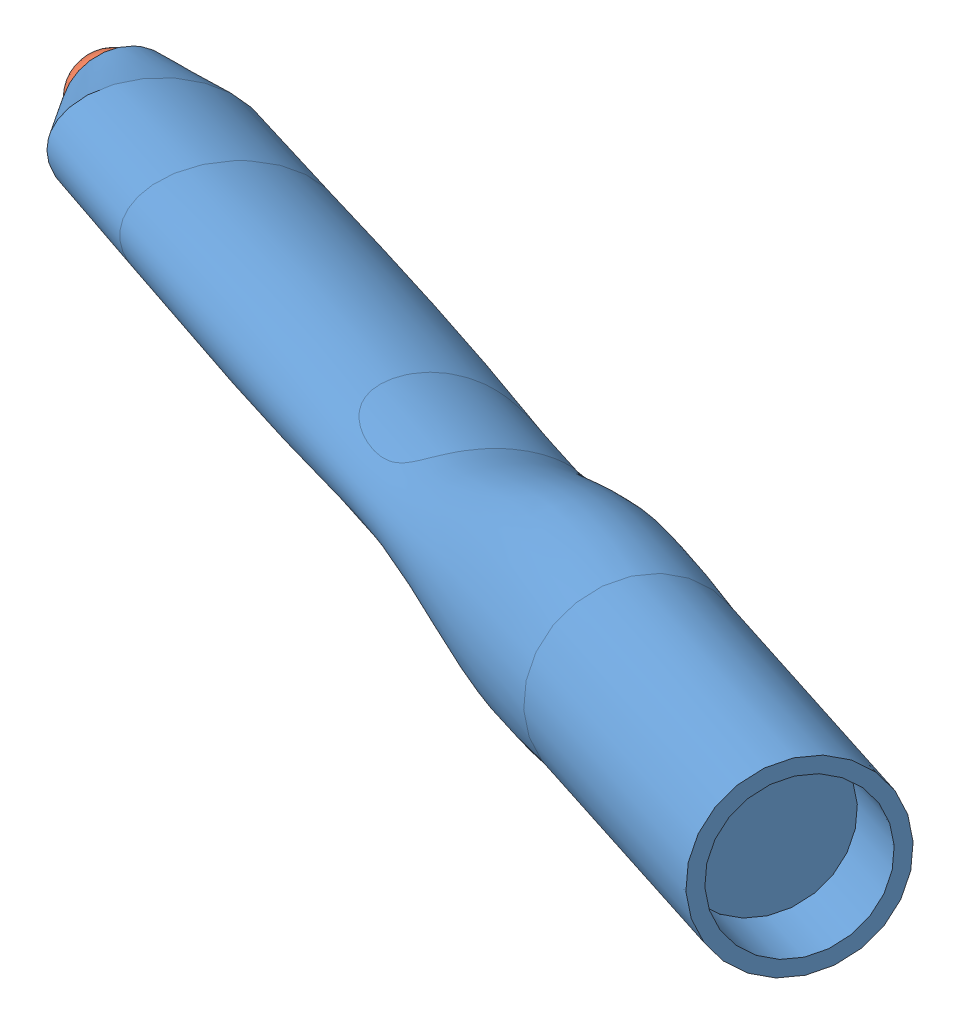
SolidWorks assembly Сборка фонарика с платой, configuration Default. Lengths in mm.
Overall size (90.97 31.39 52.87).
4 component instances, 4 part files, 6 mates.
Components (placement in the parent):
- Корпус фонарика 2-1: Корпус фонарика 2 [Default] at (-101.1891 74.0826 87.0258) x (0.421517 -0.263869 -0.867581) z (0.906373 0.152654 0.393936) size (14.16 14.28 92)
- Диод 5 мм-1: Диод 5 мм [Default] at (-160.4947 64.0942 61.2499) x (-0.418245 0.455903 0.785636) z (-0.059666 -0.876841 0.477064) size (5.3 37.5 5.3)
- Плата, окончательный вариант-2: Плата, окончательный вариант [Default] at (-90.2951 101.2878 171.0784) x (-0.906373 -0.152654 -0.393936) z (0.028492 -0.952402 0.30351) size (35.81 7.37 4.58)
- Батарейка 27А-1: Батарейка 27А [Default] at (-100.5093 74.1971 87.3213) x (0.318503 -0.85951 -0.399747) z (0.906373 0.152654 0.393936) size (7.67 7.67 30)
Mates (geometry in assembly coordinates):
- Concentric16: concentric aligned: cylinder of Корпус фонарика 2-1 through (-81.2489 77.441 95.6924) axis (-0.906373 -0.152654 -0.393936) radius 5; cylinder of Батарейка 27А-1 through (-87.8201 76.3342 92.8363) axis (-0.906373 -0.152654 -0.393936) radius 3.835
- Concentric17: concentric aligned: cylinder of Корпус фонарика 2-1 through (-147.4141 66.2972 66.9351) axis (-0.906373 -0.152654 -0.393936) radius 2.55; cylinder of Диод 5 мм-1 through (-167.8075 62.8625 58.0715) axis (-0.906373 -0.152654 -0.393936) radius 2.65
- Distance1: distance = 0.25 mm anti-aligned: plane of Батарейка 27А-1 through (-87.8201 76.3342 92.8363) normal (0.906373 0.152654 0.393936); plane of Корпус фонарика 2-1 through (-87.5935 76.3724 92.9348) normal (-0.906373 -0.152654 -0.393936)
- Coincident35: coincident anti-aligned: plane of Корпус фонарика 2-1 through (-160.1033 64.1601 61.42) normal (0.906373 0.152654 0.393936); plane of Диод 5 мм-1 through (-160.2525 61.968 62.6126) normal (-0.906373 -0.152654 -0.393936)
- Coincident36: coincident anti-aligned: plane of Корпус фонарика 2-1 through (-121.0169 72.5618 82.4655) normal (0.028492 -0.952402 0.30351); plane of Плата, окончательный вариант-2 through (-118.5445 72.8107 83.0147) normal (-0.028492 0.952402 -0.30351)
- Distance2: distance = 0.5 mm anti-aligned: plane of Плата, окончательный вариант-2 through (-151.0053 67.3436 68.9063) normal (-0.421517 0.263869 0.867581); plane of Корпус фонарика 2-1 through (-120.9884 71.6094 82.769) normal (0.421517 -0.263869 -0.867581)
